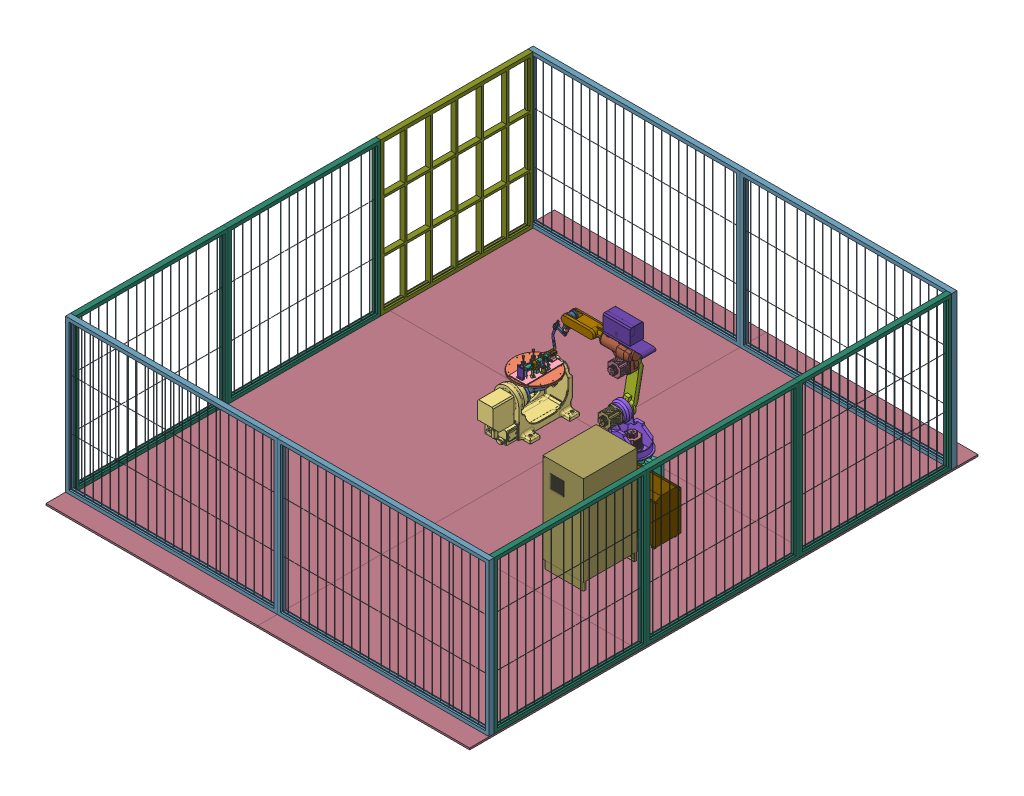
SolidWorks assembly 机器人焊接工作站总装图, configuration 默认. Lengths in mm.
Overall size (5000 1820 6000).
148 component instances, 90 part files, 30 mates.
Components (placement in the parent):
- 一轴伺服变位机-1: 一轴伺服变位机 [默认] x (-1 0 0) z (0 1 0) size (526.87 900.09 500.02)
  - 2-Axis Servo Positioner_axis1-1: 2-Axis Servo Positioner_axis1 [默认] at (91.2 313 350) x (1 0 0.000083) z (0 1 0) size (307.75 239 429)
  - 2-Axis Servo Positioner_axis2-1: 2-Axis Servo Positioner_axis2 [默认] at (91.1876 313 500) x (-0.055267 -0.998472 -0.000005) z (-0.000083 0 1) size (500 500 26)
  - 2-Axis Servo Positioner_base-1: 2-Axis Servo Positioner_base [默认] at (91.2 320 0) size (493.01 900.09 496)
- 焊接一工装总成-1: 焊接一工装总成 [默认] at (-473.6326 528.1045 352.5549) x (-0.010108 0.000001 -0.999949) z (0.999949 -0.000083 -0.010108) size (450 149.82 266.69)
  - 工装布局-1: 工装布局 [默认] at (10.7955 -18.0728 400) size (450 110 200)
  - 支撑件二-1: 支撑件二 [默认] at (-107.8852 -18.0728 400) x (0 0 1) z (-1 0 0) size (32 61 20)
  - 焊接件一-1: 焊接件一 [默认] at (313.4994 54.9272 377.8336) x (0 1 0) z (-1 0 0) size (106.25 98 315)
    - 管柱-1: 管柱 [默认] at (0 -22.1664 152.7039) size (34 34 305)
    - 法兰盘-1: 法兰盘 [默认] at (0 -22.1664 155.7039) x (-0.156434 -0.987688 0) z (0 0 -1) size (62.77 56.5 8)
    - 固定块-1: 固定块 [默认] at (0 -22.1664 462.7039) x (0 -1 0) z (1 0 0) size (80 18 91)
    - 支架一-1: 支架一 [默认] at (0 -22.1664 310.7806) x (0 -1 0) z (0 0 1) size (98 63.25 32)
    - 支架二-1: 支架二 [默认] at (0 -22.1664 182.7039) x (0 -1 0) z (0 0 1) size (98 51.76 32)
    - 支板一-1: 支板一 [默认] at (23 -22.1664 217.7039) x (0 0 1) z (0 -1 0) size (17 10 64)
    - 支板二-1: 支板二 [默认] at (23 -22.1664 421.7039) x (0 0 1) z (0 -1 0) size (17 10 92)
    - 支片-1: 支片 [默认] at (0 -22.1664 345.7806) x (0 -1 0) z (0 0 1) size (46.31 21.78 18)
    - 支片-2: 支片 [默认] at (0 -22.1664 275.7806) x (0.777146 0.62932 0) z (0 0 -1) size (46.31 21.78 18)
  - 支撑件一-1: 支撑件一 [默认] at (50.1702 -18.0728 350.9861) x (0.707107 0 0.707107) z (-0.707107 0 0.707107) size (36 92 37)
  - 支撑件二-2: 支撑件二 [默认] at (104.0197 -18.0728 400) x (0 0 -1) z (1 0 0) size (32 61 20)
  - GH-201-B-1: GH-201-B [預設] at (64.6659 73.9672 339.3188) x (0.707107 0 -0.707107) z (0.707107 0 0.707107) size (144.63 47.82 36)
    - GH-201-B_13-1: GH-201-B_13 [預設] at origin size (37 25.54 36)
    - GH-201-B_08-1: GH-201-B_08 [預設] at (-25.55 37.78 -2) x (1 0 0) z (0 -1 0) size (68.35 11.4 23.73)
    - GH-201-B_05-1: GH-201-B_05 [預設] at (-5.75 19.75 -4) x (0.886113 -0.46347 0) z (0 0 1) size (24.2 11.5 4)
    - GH-201-B_01-1: GH-201-B_01 [預設] at (-35.0495 44.2676 -2.1) x (0.987162 -0.159721 0) z (-0.159721 -0.987162 0) size (86.67 20.97 22.68)
    - GH-201-B_FC1-1: GH-201-B_FC1 [預設] at (-82.55 3.78 -2) size (16.2 44 16.2)
    - GH-201-B_FW1-1: GH-201-B_FW1 [預設] at (-82.55 37.78 -2) size (18.4 9.6 15.27)
    - GH-201-B_FW2-1: GH-201-B_FW2 [預設] at (-82.55 25.08 -2) x (1 0 0) z (0 0 -1) size (18.4 9.6 15.27)
  - 支撑件一-2: 支撑件一 [默认] at (-71.2935 -18.0728 352.1425) x (-0.707107 0 -0.707107) z (0.707107 0 -0.707107) size (36 92 37)
  - GH-201-B-2: GH-201-B [預設] at (-56.7979 73.9672 340.4753) x (0.707107 0 -0.707107) z (0.707107 0 0.707107) size (144.63 47.82 36)
    - GH-201-B_13-1: GH-201-B_13 [預設] at origin size (37 25.54 36)
    - GH-201-B_08-1: GH-201-B_08 [預設] at (-25.55 37.78 -2) x (1 0 0) z (0 -1 0) size (68.35 11.4 23.73)
    - GH-201-B_05-1: GH-201-B_05 [預設] at (-5.75 19.75 -4) x (0.886113 -0.46347 0) z (0 0 1) size (24.2 11.5 4)
    - GH-201-B_01-1: GH-201-B_01 [預設] at (-35.0495 44.2676 -2.1) x (0.987162 -0.159721 0) z (-0.159721 -0.987162 0) size (86.67 20.97 22.68)
    - GH-201-B_FC1-1: GH-201-B_FC1 [預設] at (-82.55 3.78 -2) size (16.2 44 16.2)
    - GH-201-B_FW1-1: GH-201-B_FW1 [預設] at (-82.55 37.78 -2) size (18.4 9.6 15.27)
    - GH-201-B_FW2-1: GH-201-B_FW2 [預設] at (-82.55 25.08 -2) x (1 0 0) z (0 0 -1) size (18.4 9.6 15.27)
  - GH-201-B-3: GH-201-B [預設] at (84.2467 73.9672 484.1366) x (0 0 1) z (-1 0 0) size (144.63 47.82 36)
    - GH-201-B_13-1: GH-201-B_13 [預設] at origin size (37 25.54 36)
    - GH-201-B_08-1: GH-201-B_08 [預設] at (-25.55 37.78 -2) x (1 0 0) z (0 -1 0) size (68.35 11.4 23.73)
    - GH-201-B_05-1: GH-201-B_05 [預設] at (-5.75 19.75 -4) x (0.886113 -0.46347 0) z (0 0 1) size (24.2 11.5 4)
    - GH-201-B_01-1: GH-201-B_01 [預設] at (-35.0495 44.2676 -2.1) x (0.987162 -0.159721 0) z (-0.159721 -0.987162 0) size (86.67 20.97 22.68)
    - GH-201-B_FC1-1: GH-201-B_FC1 [預設] at (-82.55 3.78 -2) size (16.2 44 16.2)
    - GH-201-B_FW1-1: GH-201-B_FW1 [預設] at (-82.55 37.78 -2) size (18.4 9.6 15.27)
    - GH-201-B_FW2-1: GH-201-B_FW2 [預設] at (-82.55 25.08 -2) x (1 0 0) z (0 0 -1) size (18.4 9.6 15.27)
  - 支撑件三-1: 支撑件三 [默认] at (86.2467 -18.0728 465.6366) size (36 92 37)
  - 支撑件四-1: 支撑件四 [默认] at (130.7955 54.9272 400) x (0 0 1) z (-1 0 0) size (100 19.36 32)
  - 支撑件五-1: 支撑件五 [默认] at (2.7187 54.9259 400) x (0 0 1) z (-1 0 0) size (100 37.36 32)
  - 支撑件七-1: 支撑件七 [默认] at (-64.7417 -18.0728 455.1147) x (0.866025 0 0.5) z (-0.5 0 0.866025) size (36 88 37)
  - 支撑件六-1: 支撑件六 [默认] at (-32.2811 54.9272 400) x (0 0 1) z (-1 0 0) size (15 78.14 20)
  - GH-201-B-4: GH-201-B [預設] at (-75.7238 69.9672 470.1361) x (-0.5 0 0.866025) z (-0.866025 0 -0.5) size (144.63 47.82 36)
    - GH-201-B_13-1: GH-201-B_13 [預設] at origin size (37 25.54 36)
    - GH-201-B_08-1: GH-201-B_08 [預設] at (-25.55 37.78 -2) x (1 0 0) z (0 -1 0) size (68.35 11.4 23.73)
    - GH-201-B_05-1: GH-201-B_05 [預設] at (-5.75 19.75 -4) x (0.886113 -0.46347 0) z (0 0 1) size (24.2 11.5 4)
    - GH-201-B_01-1: GH-201-B_01 [預設] at (-35.0495 44.2676 -2.1) x (0.987162 -0.159721 0) z (-0.159721 -0.987162 0) size (86.67 20.97 22.68)
    - GH-201-B_FC1-1: GH-201-B_FC1 [預設] at (-82.55 3.78 -2) size (16.2 44 16.2)
    - GH-201-B_FW1-1: GH-201-B_FW1 [預設] at (-82.55 37.78 -2) size (18.4 9.6 15.27)
    - GH-201-B_FW2-1: GH-201-B_FW2 [預設] at (-82.55 25.08 -2) x (1 0 0) z (0 0 -1) size (18.4 9.6 15.27)
  - 支撑件八-1: 支撑件八 [默认] at (37.7189 54.9272 400) x (0 0.777146 -0.62932) z (1 0 0) size (46.2 37.09 20)
  - GH-36070-1: GH-36070 [預設] at (38.0052 43.9272 449.5811) x (0 0 1) z (-1 0 0) size (135.91 23 41)
    - GH-36070_13-1: GH-36070_13 [預設] at origin size (57.5 23 41)
    - GH-36070_33-1: GH-36070_33 [預設] at origin size (37.22 7.99 7.99)
    - GH-36070_N1-1: GH-36070_N1 [預設] at origin size (4 9.24 8)
    - GH-36070_SA1-1: GH-36070_SA1 [預設] at origin size (19.5 9.24 8)
    - GH-36070_05-1: GH-36070_05 [預設] at origin size (25.91 8.33 10)
    - GH-36070_01-1: GH-36070_01 [預設] at origin size (79.52 13.85 25.4)
  - 支撑件九-1: 支撑件九 [默认] at (38.0052 -18.0728 479.5811) size (41 62 40)
  - 支撑件十-1: 支撑件十 [默认] at (-149.2045 -18.0728 400) x (0 1 0) z (-1 0 0) size (106 70 25)
  - TN_16x10_S__0_-1: TN_16x10_S__0_ [TN-16x10-S (0)] at (191.5841 44.3272 400) x (1 0 0) z (0 -1 0) size (78 54.3 21.2)
    - TN16_10___10_b-1: TN16_10___10_b [默认] x (1 0 0) z (0 1 0) size (70.5 21.2 54.3)
    - TN16_10_fp-1: TN16_10_fp [默认] at (-15 0 -0.6) x (1 0 0) z (0 1 0) size (8 20 53)
    - TN_16_1010_r-1: TN_16_1010_r [默认] at (-8 -12 -10.6) x (1 0 0) z (0 0 -1) size (65.6 15.6 15.6)
    - TN_16_1010_r-2: TN_16_1010_r [默认] at (-8 12 -10.6) x (1 0 0) z (0 0 -1) size (65.6 15.6 15.6)
    - TN16s-1: TN16s [默认] at (-14.4 12 -10.6) x (1 0 0) z (0 1 0) size (12.5 7 7)
    - TN16s-2: TN16s [默认] at (-14.4 -12 -10.6) x (1 0 0) z (0 1 0) size (12.5 7 7)
  - 支撑件十一-1: 支撑件十一 [默认] at (223.0841 -18.0728 400) x (0 0 1) z (-1 0 0) size (54 62.4 63)
  - 支撑件十二-1: 支撑件十二 [默认] at (158.5841 54.9272 400) x (0 -0.156434 0.987688) z (1 0 0) size (64 64 18)
- RB08-1: RB08 [默认] at (1044.2533 0 301.307) x (1 0 0) z (0 1 0) size (1065.83 389.5 1320.66)
  - 底座-1: 底座 [默认] at origin size (433 340 242)
  - 大臂-1: 大臂 [默认] at (-170 75 530) x (0.161371 0 0.986894) z (0 1 0) size (730 190 120)
  - 转盘-1: 转盘 [默认] at (0 0 217) x (-1 0 0) z (0 0 1) size (470 385 420.5)
  - 小臂-1: 小臂 [默认] at (-293.6325 0 1237.6606) x (-1 0 0) z (0 -0.999953 -0.009736) size (472 150 150)
  - 手腕-1: 手腕 [默认] at (-719.6325 0 1237.6606) x (-0.934001 -0.003478 0.357254) z (0 0.999953 0.009736) size (94 157 73)
  - 箱体-1: 箱体 [默认] at (-4.6325 0 1237.6606) x (0 1 0) z (1 0 0) size (246 343 358)
  - 电机2-1: 电机2 [默认] at (-170 -34 530) x (-1 0 0) z (0 1 0) size (150 150 239)
  - 电机1-1: 电机1 [默认] at (0 0 288) x (1 0 0) z (0 0 -1) size (150 150 211)
  - 电机1-2: 电机1 [默认] at (-79.6325 -36 1082.6606) x (1 0 0) z (0 1 0) size (150 150 211)
- 31度鵝頸，支架100.5L-1: 31度鵝頸，支架100.5L [默认] at (278.7071 1116.7088 301.4518) x (0 -0.009736 0.999953) z (-0.357271 -0.933956 -0.009093) size (70 159.03 372.5)
  - 31度鵝頸，支架100.5L-Part-1-1: 31度鵝頸，支架100.5L-Part-1 [默认] at (-1.3223 63.2513 288.8466) x (1 0 0) z (0 -0.857167 -0.515038) size (20 65.51 20)
  - 31度鵝頸，支架100.5L-Part-2-1: 31度鵝頸，支架100.5L-Part-2 [默认] at (-1.3223 48.8303 312.8473) x (0 -0.515038 0.857167) z (-0.857167 0.441474 0.265264) size (40.5 8.7 8.7)
  - 31度鵝頸，支架100.5L-Part-3-1: 31度鵝頸，支架100.5L-Part-3 [默认] at (-1.3223 56.2983 300.4183) x (1 0 0) z (0 -0.857167 -0.515038) size (15.5 21 15.5)
  - 31度鵝頸，支架100.5L-Part-4-1: 31度鵝頸，支架100.5L-Part-4 [默认] at (-1.3223 63.7664 287.9894) x (0.857167 -0.441474 -0.265264) z (0 -0.515038 0.857167) size (20 20 1)
  - 31度鵝頸，支架100.5L-Part-4-2: 31度鵝頸，支架100.5L-Part-4 [默认] at (-1.3223 63.2513 288.8466) x (1 0 0) z (0 0.515038 -0.857167) size (20 20 1)
  - 31度鵝頸，支架100.5L-Part-5-1: 31度鵝頸，支架100.5L-Part-5 [默认] at (-1.3223 76.3848 266.9888) x (0 -0.515038 0.857167) z (-0.857167 0.441474 0.265264) size (38 20 20)
  - 31度鵝頸，支架100.5L-Part-6-1: 31度鵝頸，支架100.5L-Part-6 [默认] at (-1.3223 76.3848 266.9888) x (0 -0.515038 0.857167) z (-0.857167 0.441474 0.265264) size (33.02 20 20)
  - 31度鵝頸，支架100.5L-Part-7-1: 31度鵝頸，支架100.5L-Part-7 [默认] at (-1.3223 44.9675 319.276) x (0 0.515038 -0.857167) z (0.857167 0.441474 0.265264) size (80 14 16)
  - 31度鵝頸，支架100.5L-Part-8-1: 31度鵝頸，支架100.5L-Part-8 [默认] at (-1.3223 100.8266 121.034) x (0 0 -1) z (1 0 0) size (2 12 12)
  - 31度鵝頸，支架100.5L-Part-9-1: 31度鵝頸，支架100.5L-Part-9 [默认] at (-1.3223 0.3266 10.634) x (0 0 -1) z (-1 0 0) size (20 70 70)
  - 31度鵝頸，支架100.5L-Part-10-1: 31度鵝頸，支架100.5L-Part-10 [默认] at (-16.0584 25.8771 1.634) x (-1 0 0) z (0 0 1) size (7 7 19)
  - 31度鵝頸，支架100.5L-Part-10-2: 31度鵝頸，支架100.5L-Part-10 [默认] at (13.4416 25.8771 1.634) x (-1 0 0) z (0 0 1) size (7 7 19)
  - 31度鵝頸，支架100.5L-Part-10-3: 31度鵝頸，支架100.5L-Part-10 [默认] at (-30.8084 0.3294 1.634) x (-1 0 0) z (0 0 1) size (7 7 19)
  - 31度鵝頸，支架100.5L-Part-10-4: 31度鵝頸，支架100.5L-Part-10 [默认] at (13.4416 -25.2184 1.634) x (-1 0 0) z (0 0 1) size (7 7 19)
  - 31度鵝頸，支架100.5L-Part-10-5: 31度鵝頸，支架100.5L-Part-10 [默认] at (-16.0584 -25.2184 1.634) x (-1 0 0) z (0 0 1) size (7 7 19)
  - 31度鵝頸，支架100.5L-Part-11-1: 31度鵝頸，支架100.5L-Part-11 [默认] at (-1.3223 0.3266 119.534) x (0.923728 0.383049 0) z (0 0 -1) size (8.5 8.5 13.05)
  - 31度鵝頸，支架100.5L-Part-12-1: 31度鵝頸，支架100.5L-Part-12 [默认] at (-1.3223 0.3266 114.534) x (-0.923728 -0.383049 0) z (0 0 -1) size (19.5 19.5 2)
  - 31度鵝頸，支架100.5L-Part-13-1: 31度鵝頸，支架100.5L-Part-13 [默认] at (10.6777 113.8266 135.234) x (0.381849 0 0.924225) z (0 -1 0) size (10 10 26.16)
  - 31度鵝頸，支架100.5L-Part-13-2: 31度鵝頸，支架100.5L-Part-13 [默认] at (14.1777 12.3266 102.534) x (0 -0.924225 -0.381849) z (-1 0 0) size (10 10 26.16)
  - 31度鵝頸，支架100.5L-Part-14-1: 31度鵝頸，支架100.5L-Part-14 [默认] at (-19.8223 113.3266 105.034) x (1 0 0) z (0 -1 0) size (10 10 28.16)
  - 31度鵝頸，支架100.5L-Part-14-2: 31度鵝頸，支架100.5L-Part-14 [默认] at (17.1777 114.3266 105.034) x (1 0 0) z (0 -1 0) size (10 10 28.16)
  - 31度鵝頸，支架100.5L-Part-15-1: 31度鵝頸，支架100.5L-Part-15 [默认] at (-1.3223 -19.6734 117.534) x (-1 0 0) z (0 0 -1) size (50 120 25)
  - 31度鵝頸，支架100.5L-Part-16-1: 31度鵝頸，支架100.5L-Part-16 [默认] at (-1.3223 -19.6734 117.534) x (-1 0 0) z (0 0 -1) size (50 20 25)
  - 31度鵝頸，支架100.5L-Part-17-1: 31度鵝頸，支架100.5L-Part-17 [默认] at (-1.3223 -19.6734 117.534) x (-1 0 0) z (0 0 -1) size (12 12 12)
  - 31度鵝頸，支架100.5L-Part-18-1: 31度鵝頸，支架100.5L-Part-18 [默认] at (-1.3223 0.3266 53.134) x (1 0 0) z (0 -1 0) size (50 38.5 50)
  - 31度鵝頸，支架100.5L-Part-19-1: 31度鵝頸，支架100.5L-Part-19 [默认] at (-1.3223 -8.6734 110.134) x (1 0 0) z (0 1 0) size (3 15.7 3)
  - 31度鵝頸，支架100.5L-Part-20-1: 31度鵝頸，支架100.5L-Part-20 [默认] at (-1.3223 0.3266 50.534) x (0 0 1) z (-1 0 0) size (61.8 31 31)
  - 31度鵝頸，支架100.5L-Part-21-1: 31度鵝頸，支架100.5L-Part-21 [默认] at (-1.3223 20.3266 59.134) x (1 0 0) z (0 1 0) size (6.95 6.95 7)
  - 31度鵝頸，支架100.5L-Part-21-2: 31度鵝頸，支架100.5L-Part-21 [默认] at (-1.3223 -19.6734 59.134) x (1 0 0) z (0 -1 0) size (6.95 6.95 7)
  - 31度鵝頸，支架100.5L-Part-21-3: 31度鵝頸，支架100.5L-Part-21 [默认] at (-21.3223 0.3266 59.134) x (0 0 1) z (-1 0 0) size (6.95 6.95 7)
  - 31度鵝頸，支架100.5L-Part-21-4: 31度鵝頸，支架100.5L-Part-21 [默认] at (18.6777 0.3266 59.134) x (0 0 -1) z (1 0 0) size (6.95 6.95 7)
  - 31度鵝頸，支架100.5L-Part-22-1: 31度鵝頸，支架100.5L-Part-22 [默认] at (-8.8223 24.8266 49.634) size (5.7 9.6 5.7)
  - 31度鵝頸，支架100.5L-Part-22-2: 31度鵝頸，支架100.5L-Part-22 [默认] at (6.1777 24.8266 49.634) size (5.7 9.6 5.7)
  - 31度鵝頸，支架100.5L-Part-22-3: 31度鵝頸，支架100.5L-Part-22 [默认] at (-8.8223 24.8266 7.634) size (5.7 9.6 5.7)
  - 31度鵝頸，支架100.5L-Part-22-4: 31度鵝頸，支架100.5L-Part-22 [默认] at (6.1777 24.8266 7.634) size (5.7 9.6 5.7)
  - 31度鵝頸，支架100.5L-Part-23-1: 31度鵝頸，支架100.5L-Part-23 [默认] at (-1.3223 0.3266 65.634) x (-0.707107 -0.707107 0) z (0 0 -1) size (42 42 1)
  - 31度鵝頸，支架100.5L-Part-24-1: 31度鵝頸，支架100.5L-Part-24 [默认] at (-1.3223 0.3266 65.634) x (-0.707107 -0.707107 0) z (0 0 -1) size (42 42 1)
  - 31度鵝頸，支架100.5L-Part-25-1: 31度鵝頸，支架100.5L-Part-25 [默认] at (-1.3223 0.3266 53.634) size (42 42 11)
  - 31度鵝頸，支架100.5L-Part-26-1: 31度鵝頸，支架100.5L-Part-26 [默认] at (-1.3223 0.3266 -1.366) x (0 0 -1) z (1 0 0) size (14.5 70 70)
  - 31度鵝頸，支架100.5L-Part-27-1: 31度鵝頸，支架100.5L-Part-27 [默认] at (-1.3223 0.3266 -0.366) size (47 47 60)
  - 31度鵝頸，支架100.5L-Part-28-1: 31度鵝頸，支架100.5L-Part-28 [默认] at (-1.3223 0.3266 -0.366) size (21.17 11.67 48)
  - 31度鵝頸，支架100.5L-Part-29-1: 31度鵝頸，支架100.5L-Part-29 [默认] at (-1.3223 0.3266 -0.366) size (21 1.5 48)
  - 31度鵝頸，支架100.5L-Part-30-1: 31度鵝頸，支架100.5L-Part-30 [默认] at (-1.3223 109.3266 144.534) x (-1 0 0) z (0 -1 0) size (3 12.5 3)
  - 31度鵝頸，支架100.5L-Part-31-1: 31度鵝頸，支架100.5L-Part-31 [默认] at (-1.3223 100.8266 121.034) x (0 0 -1) z (1 0 0) size (127.05 42.81 19)
  - 31度鵝頸，支架100.5L-Part-32-1: 31度鵝頸，支架100.5L-Part-32 [默认] at (-1.3223 100.8266 121.034) x (0 0 -1) z (1 0 0) size (148.04 38.42 16.86)
  - 31度鵝頸，支架100.5L-Part-33-1: 31度鵝頸，支架100.5L-Part-33 [默认] at (-1.3223 100.8266 120.534) x (-0.546944 0.837169 0) z (0 0 -1) size (34 34 55)
  - 31度鵝頸，支架100.5L-Part-34-1: 31度鵝頸，支架100.5L-Part-34 [默认] at (-1.3223 100.8266 145.534) x (0 1 0) z (-1 0 0) size (33 105 33)
- RB08电控柜-1: RB08电控柜 [默认] at (1737.1297 0 1483.7342) x (0 0 1) z (-1 0 0) size (635 1150 552)
- 水泥地面-1: 水泥地面 [默认] at (-2103.4719 0 4072.4085) size (5000 20 6000)
- 安全护栏2500x1800-1: 安全护栏2500x1800 [默认] at (-853.4719 0 -1647.5915) size (2500 1800 60)
- 安全护栏2500x1800-2: 安全护栏2500x1800 [默认] at (1646.5281 0 -1647.5915) size (2500 1800 60)
- 安全护栏1800x1800-1: 安全护栏1800x1800 [默认] at (2866.5281 0 -717.5915) x (0 0 1) z (-1 0 0) size (1800 1800 60)
- 安全护栏1800x1800-2: 安全护栏1800x1800 [默认] at (2866.5281 0 1082.4085) x (0 0 1) z (-1 0 0) size (1800 1800 60)
- 安全护栏1800x1800-3: 安全护栏1800x1800 [默认] at (2866.5281 0 2882.4085) x (0 0 1) z (-1 0 0) size (1800 1800 60)
- 安全护栏2500x1800-4: 安全护栏2500x1800 [默认] at (-853.4719 0 3812.4085) size (2500 1800 60)
- 安全护栏2500x1800-6: 安全护栏2500x1800 [默认] at (1646.5281 0 3812.4085) size (2500 1800 60)
- 安全护栏1800x1800-4: 安全护栏1800x1800 [默认] at (-2073.4719 0 2882.4085) x (0 0 1) z (-1 0 0) size (1800 1800 60)
- 安全护栏1800x1800-5: 安全护栏1800x1800 [默认] at (-2073.4719 0 1082.4085) x (0 0 1) z (-1 0 0) size (1800 1800 60)
- 安全门-1: 安全门 [默认] at (-2073.4719 0 -717.5915) x (0 0 1) z (-1 0 0) size (1800 1800 60)
- 送丝机-1: 送丝机 [默认] at (943.7354 1364.6606 306.307) x (0 0 1) z (-1 0 0) size (162.2 246.99 472.57)
- 焊机-1: 焊机 [默认] at (1686.7696 40 816.6527) x (0 0 1) z (-1 0 0) size (300 540 600)
Mates (geometry in assembly coordinates):
- 重合4: coincident anti-aligned: plane of 一轴伺服变位机-1/2-Axis Servo Positioner_axis2-1 through (-326.0003 500.0195 50.6697) normal (0.000083 1 0); plane of 焊接一工装总成-1/工装布局-1 through (-73.7645 499.9986 337.7167) normal (-0.000083 -1 0)
- 同心1: concentric aligned: cylinder of RB08-1/手腕-1 through (286.7501 1138.6612 300.3432) axis (-0.357271 -0.933956 -0.009093) radius 25; cylinder of 31度鵝頸，支架100.5L-1/31度鵝頸，支架100.5L-Part-26-1 through (282.2842 1126.9868 300.2295) axis (-0.357271 -0.933956 -0.009093) radius 12.45
- 重合7: coincident anti-aligned: plane of RB08-1/手腕-1 through (285.321 1134.9254 300.3068) normal (-0.357271 -0.933956 -0.009093); plane of 31度鵝頸，支架100.5L-1/31度鵝頸，支架100.5L-Part-26-1 through (273.6927 1139.3732 300.3501) normal (0.357271 0.933956 0.009093)
- 平行2: parallel aligned: plane of RB08-1/手腕-1 through (334.3903 1130.4297 263.7613) normal (0 0.009736 -0.999953); plane of 31度鵝頸，支架100.5L-1/31度鵝頸，支架100.5L-Part-28-1 through (247.7925 1123.6875 289.6969) normal (0 0.009736 -0.999953)
- 重合8: coincident aligned: plane of RB08-1/底座-1 through (874.2533 0 471.307) normal (0 -1 0); plane of RB08电控柜-1 through (1737.1297 0 1483.7342) normal (0 -1 0)
- 重合9: coincident anti-aligned: plane of 一轴伺服变位机-1/2-Axis Servo Positioner_base-1 through (-341.2 0 496) normal (0 -1 0); plane of assembly through (0 0 0) normal (0 1 0)
- 重合10: coincident aligned: plane of 一轴伺服变位机-1/2-Axis Servo Positioner_base-1 through (0 156 651) normal (1 0 0); plane of assembly through (0 0 0) normal (1 0 0)
- 重合11: coincident anti-aligned: plane of 一轴伺服变位机-1/2-Axis Servo Positioner_base-1 through (-1.2 442 0) normal (0 0 -1); plane of assembly through (0 0 0) normal (0 0 1)
- 重合12: coincident aligned: plane of 一轴伺服变位机-1/2-Axis Servo Positioner_base-1 through (14.8 0 496) normal (0 -1 0); plane of RB08-1/底座-1 through (874.2533 0 471.307) normal (0 -1 0)
- 重合13: coincident aligned: plane of RB08-1/底座-1 through (874.2533 0 471.307) normal (0 -1 0); plane of RB08电控柜-1 through (1737.1297 0 1483.7342) normal (0 -1 0)
- 重合15: coincident anti-aligned: plane of RB08-1/底座-1 through (874.2533 0 471.307) normal (0 -1 0); plane of 水泥地面-1 through (396.5281 0 2072.4085) normal (0 1 0)
- 重合16: coincident anti-aligned: plane of 水泥地面-1 through (-2103.4719 0 72.4085) normal (0 1 0); plane of 安全护栏2500x1800-1 through (396.5281 0 -1677.5915) normal (0 -1 0)
- 距离1: distance = 250 mm aligned: plane of 水泥地面-1 through (-2103.4719 -20 -1927.5915) normal (0 0 -1); plane of 安全护栏2500x1800-1 through (396.5281 0 -1677.5915) normal (0 0 -1)
- 重合18: coincident aligned: plane of 水泥地面-1 through (-2103.4719 -20 72.4085) normal (-1 0 0); plane of 安全护栏2500x1800-1 through (-2103.4719 0 -1647.5915) normal (-1 0 0)
- 重合19: coincident anti-aligned: plane of 安全护栏2500x1800-2 through (2896.5281 0 -1617.5915) normal (0 0 1); plane of 安全护栏1800x1800-1 through (2866.5281 0 -1617.5915) normal (0 0 -1)
- 重合20: coincident aligned: plane of 安全护栏2500x1800-2 through (2896.5281 0 -1647.5915) normal (1 0 0); plane of 安全护栏1800x1800-1 through (2896.5281 0 182.4085) normal (1 0 0)
- 重合21: coincident anti-aligned: plane of 水泥地面-1 through (396.5281 0 72.4085) normal (0 1 0); plane of 安全护栏1800x1800-1 through (2896.5281 0 182.4085) normal (0 -1 0)
- 重合25: coincident anti-aligned: plane of 安全护栏2500x1800-2 through (2896.5281 0 -1617.5915) normal (0 0 1); plane of 安全护栏1800x1800-1 through (2866.5281 0 -1617.5915) normal (0 0 -1)
- 重合26: coincident anti-aligned: plane of 安全护栏2500x1800-2 through (2896.5281 0 -1617.5915) normal (0 0 1); plane of 安全护栏1800x1800-1 through (2866.5281 0 -1617.5915) normal (0 0 -1)
- 重合31: coincident anti-aligned: plane of 安全护栏2500x1800-4 through (396.5281 0 3782.4085) normal (0 0 -1); plane of 安全护栏1800x1800-4 through (-2073.4719 0 3782.4085) normal (0 0 1)
- 重合32: coincident aligned: plane of 安全护栏2500x1800-4 through (-2103.4719 0 3812.4085) normal (-1 0 0); plane of 安全护栏1800x1800-4 through (-2103.4719 0 3782.4085) normal (-1 0 0)
- 重合34: coincident aligned: plane of 安全护栏2500x1800-4 through (396.5281 1800 3782.4085) normal (0 1 0); plane of 安全护栏1800x1800-4 through (-2043.4719 1800 3782.4085) normal (0 1 0)
- 重合35: coincident aligned: line of 安全护栏2500x1800-1 through (-2103.4719 1800 -1617.5915) axis (0 -1 0); line of 安全门-1 through (-2103.4719 1800 -1617.5915) axis (0 -1 0)
- 重合36: coincident anti-aligned: plane of 水泥地面-1 through (-2103.4719 0 72.4085) normal (0 1 0); plane of 安全门-1 through (-2043.4719 0 182.4085) normal (0 -1 0)
- 角度1: planar angle = 0 rad aligned: plane of 安全门-1 through (-2103.4719 1800 182.4085) normal (-1 0 0); plane of 安全护栏2500x1800-1 through (-2103.4719 0 -1647.5915) normal (-1 0 0)
- 同心2: concentric anti-aligned: cylinder of RB08-1/箱体-1 through (831.1208 1320.6606 276.307) axis (0 1 0) radius 2.5; cylinder of 送丝机-1 through (831.1208 1350.6606 276.307) axis (0 -1 0) radius 4
- 同心3: concentric anti-aligned: cylinder of RB08-1/箱体-1 through (971.1208 1320.6606 336.307) axis (0 1 0) radius 2.5; cylinder of 送丝机-1 through (971.1208 1350.6606 336.307) axis (0 -1 0) radius 4
- 重合37: coincident anti-aligned: plane of RB08-1/箱体-1 through (971.1208 1320.6606 336.307) normal (0 1 0); plane of 送丝机-1 through (943.7354 1320.6606 306.307) normal (0 -1 0)
- 重合38: coincident anti-aligned: plane of 水泥地面-1 through (396.5281 0 72.4085) normal (0 1 0); plane of 焊机-1 through (1934.3709 0 696.9463) normal (0 -1 0)
- 平行3: parallel anti-aligned: plane of 水泥地面-1 through (396.5281 -20 4072.4085) normal (0 0 1); plane of 焊机-1 through (1386.7696 540 666.6527) normal (0 0 -1)
